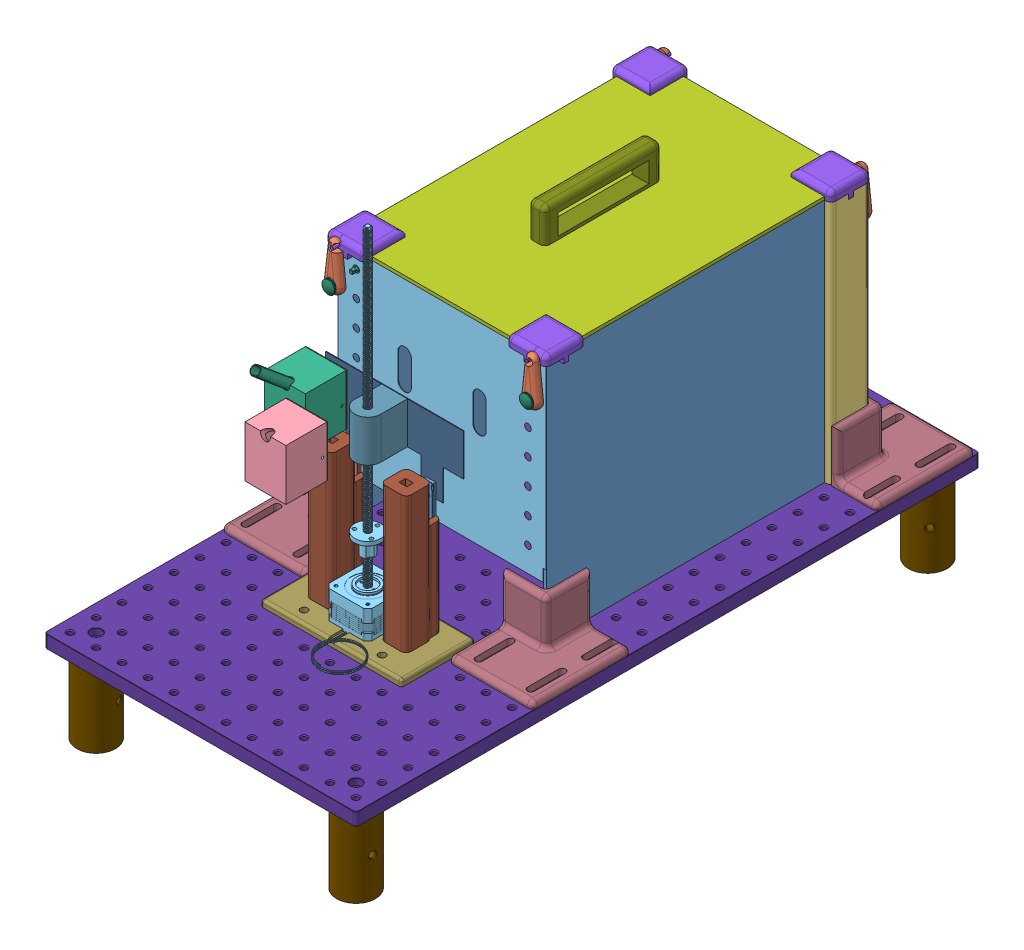
SolidWorks assembly Cage_model, configuration Default. Lengths in mm.
Overall size (306.09 428.48 610.88).
37 component instances, 27 part files, 73 mates.
Components (placement in the parent):
- Cage_acryllic_main-1: Cage_acryllic_main [Default] at (116.4275 -22.4186 -541.0136) size (203.2 239 304.17)
- Locking Mechanism^Cage_model-1: Locking Mechanism^Cage_model [Default] at (119.1314 -13.6836 -491.0988) x (0.989545 0 -0.144222) z (0.144222 0 0.989545) size (209.18 47.14 36.28) (virtual)
- Rear Legs^Cage_model-1: Rear Legs^Cage_model [Default] at (116.4275 -20.4186 -541.0136) x (0 0 -1) z (1 0 0) size (39.08 239 215.9) (virtual)
- Copy of Copy of Tube_Housing^Cage_model-1: Copy of Copy of Tube_Housing^Cage_model [Default] at (-6032.3573 5923.2833 -81.4233) size (40 50 40) (virtual)
- Stainless_steel_faceplate^Cage_model-1: Stainless_steel_faceplate^Cage_model [Default] at (116.4275 -20.4186 -236.8386) x (1 0 0) z (0 0 -1) size (203.2 188.94 0.61)
- Copy of Tube_Housing^Cage_model-2: Copy of Tube_Housing^Cage_model [Default] at (-6110.9268 5878.9507 -178.946) size (40 77.55 71.62) (virtual)
- cage top^Cage_model-1: cage top^Cage_model [Default] at (115.7745 -70.1218 -538.1595) size (203.2 3.18 304.78) (virtual)
- Top Securing Mechanisms-1: Top Securing Mechanisms [Default] at (-397.5627 136.2654 -668.6884) x (0 0 -1) z (0 1 0) size (45.43 215.9 14.36)
- doorMotorStand ^Cage_model-1: doorMotorStand ^Cage_model [Default] at (-254.8675 208.1203 679.8373) x (1 0 0) z (0 1 0) (virtual)
- Front legs^Cage_model-2: Front legs^Cage_model [Default] at (-86.7725 -20.4186 -236.229) x (0 0 1) z (-1 0 0) size (39.36 239 215.9) (hidden, virtual)
- Locking Mechanism^Cage_model-2: Locking Mechanism^Cage_model [Default] at (-90.3528 -13.1056 -286.1438) x (-0.989536 0.004347 0.144222) z (-0.144221 0.000634 -0.989545) size (209.18 47.14 36.28) (virtual)
- Top Securing Mechanisms-3: Top Securing Mechanisms [Default] at (427.2177 136.2654 -108.5542) x (0 0 1) z (0 1 0) size (45.43 215.9 14.36)
- Housing Door^Cage_model-1: Housing Door^Cage_model [Default] at (-6032.3573 5923.2833 -73.9233) x (-1 0 0) z (0 0 -1) size (40 50 0.61) (virtual)
- Door-2: Door [Default] at (467.6811 -160.8236 14.8493) x (0.996569 0.000281 -0.082761) z (-0.082738 -0.020299 -0.996365) size (134.22 71.08 12.57)
- Part6^Cage_model-4: Part6^Cage_model [Default] at (95.2928 -92.5203 546.9194) size (25.4 134.62 36.77) (virtual)
- Mounting Bracket nozzle holder-1: Mounting Bracket nozzle holder [Default] at (14.5275 -22.4186 -254) x (0 0 1) z (0 1 0) size (71.72 137.74 6.35)
- Angle Bracket_Leg Securing Mechanism-1: Angle Bracket_Leg Securing Mechanism [Default] at (156.2683 -22.4186 6.3564) x (1 0 0) z (0 1 0) size (304.2 433 50.8)
- Part6^Cage_model-5: Part6^Cage_model [Default] at (168.4928 -92.5203 546.8933) size (25.4 134.62 36.77) (virtual)
- Housing Door^Cage_model-2: Housing Door^Cage_model [Default] at (-6110.9268 5878.9507 -171.446) x (-1 0 0) z (0 0 -1) size (40 50 0.61) (virtual)
- Linear Motion Attachment Housing -2: Linear Motion Attachment Housing  [Default] at (68.2215 2233.7833 0) size (25.4 40.64 38.78)
- Part9^Cage_model-2: Part9^Cage_model [Default] at (239.0332 27.7971 -233.529) x (0.96536 0.260922 0) z (0 0 1) size (12.58 12.58 14.5) (virtual)
- Part9^Cage_model-1: Part9^Cage_model [Default] at (-93.8399 -16.6938 -233.529) x (0.891037 -0.453931 0) z (0 0 1) size (12.58 12.58 14.5) (virtual)
- Top Handle^Cage_model-1: Top Handle^Cage_model [Default] at (-0.1143 219.7614 179.188) x (1 0 0) z (0 1 0) size (16.56 114.3 33) (virtual)
- locking_mechanism^Cage_model-1: locking_mechanism^Cage_model [Default] at (0 0 310.525) (virtual)
- MB1224-Solidworks-1: MB1224-Solidworks [Default] at (14.5275 -35.1186 -304.8) x (0 0 1) z (-1 0 0) size (609.6 12.7 304.8)
- P3-Solidworks-1: P3-Solidworks [Web Part] at (-112.4725 -73.2186 -25.4) x (0.255609 0 0.96678) z (-0.96678 0 0.255609) size (37.74 76.2 37.94)
- P3-Solidworks-2: P3-Solidworks [Web Part] at (141.5275 -73.2186 -25.4) x (0.123275 0 -0.992373) z (0.992373 0 0.123275) size (37.74 76.2 37.94)
- P3-Solidworks-3: P3-Solidworks [Web Part] at (141.5275 -73.2186 -584.2) x (0.652104 0 -0.75813) z (0.75813 0 0.652104) size (37.74 76.2 37.94)
- P3-Solidworks-4: P3-Solidworks [Web Part] at (-112.4725 -73.2186 -584.2) x (-0.90982 0 0.415002) z (-0.415002 0 -0.90982) size (37.74 76.2 37.94)
- 3363N14_Miniature Pass-Through Drawer Slides-1: 3363N14_Miniature Pass-Through Drawer Slides [3363N14] at (51.1275 42.2414 -183.1224) x (0 1 0) z (0 0 -1) size (99.77 16 6)
- 3363N14_Miniature Pass-Through Drawer Slides (1)-1: 3363N14_Miniature Pass-Through Drawer Slides (1) [3363N14] at (-22.0725 42.2414 -183.0962) x (0 1 0) z (0 0 -1) size (99.77 16 6)
- 91028A658_JIS Hex Nut-1: 91028A658_JIS Hex Nut [91028A658] at (78.0275 -37.1186 -139.7) x (-0.777282 0 -0.629153) z (0.629153 0 -0.777282) size (8 4.57 9.24)
- 91028A658_JIS Hex Nut-4: 91028A658_JIS Hex Nut [91028A658] at (103.4275 -37.1186 -114.3) x (-0.799453 0 0.600729) z (-0.600729 0 -0.799453) size (8 4.57 9.24)
- LA1700-Solidworks-1: LA1700-Solidworks [Default] at (60.0219 191.9413 -69.6876) x (0 -0.690695 0.723146) z (-1 0 0) size (6 6 1.79)
- 8677N21_Stepper Motor with Linear Actuation-1: 8677N21_Stepper Motor with Linear Actuation [8677N21] at (14.5275 163.7634 -163.8403) x (0 -1 0) z (1 0 0) size (339.67 87.09 59.64)
- 91430A226_18-8 Stainless Steel Slotted Flat Head Screws (2)-1: 91430A226_18-8 Stainless Steel Slotted Flat Head Screws (2) [91430A226] at (-69.0425 51.5814 -357.659) x (0 0 1) z (0.105467 0.994423 0) size (16.28 7.5 7.43)
- 91430A226_18-8 Stainless Steel Slotted Flat Head Screws (2)-2: 91430A226_18-8 Stainless Steel Slotted Flat Head Screws (2) [91430A226] at (-69.0425 201.5814 -238.8065) x (0 0 1) z (-0.058058 -0.998313 0) size (16.28 7.5 7.43)
Mates (geometry in assembly coordinates):
- Front right post alignment to breadboard: coincident anti-aligned: plane of MB1224-Solidworks-1 through (-134.8725 -35.1186 -606.6) normal (0 -1 0); plane of P3-Solidworks-1 through (-112.4725 -35.1186 -25.4) normal (0 1 0)
- Rear left post hole alignement : concentric anti-aligned: circle of MB1224-Solidworks-1; circle of P3-Solidworks-3
- Rear right post hole alignment: concentric anti-aligned: circle of MB1224-Solidworks-1; circle of P3-Solidworks-4
- rear left post to breadboard: coincident anti-aligned: plane of MB1224-Solidworks-1 through (-134.8725 -35.1186 -606.6) normal (0 -1 0); plane of P3-Solidworks-3 through (141.5275 -35.1186 -584.2) normal (0 1 0)
- rear right post to breadboard: coincident anti-aligned: plane of MB1224-Solidworks-1 through (-134.8725 -35.1186 -606.6) normal (0 -1 0); plane of P3-Solidworks-4 through (-112.4725 -35.1186 -584.2) normal (0 1 0)
- Front right post hole alignment: concentric anti-aligned: circle of MB1224-Solidworks-1; circle of P3-Solidworks-1
- Coincident110: coincident anti-aligned: plane of Cage_acryllic_main-1 through (116.4275 -22.4186 -236.8386) normal (0 0 1); plane of Stainless_steel_faceplate^Cage_model-1 through (116.4275 -20.4186 -236.8386) normal (0 0 -1)
- Coincident111: coincident aligned: plane of Cage_acryllic_main-1 through (116.4275 -22.4186 -537.8386) normal (1 0 0); plane of Stainless_steel_faceplate^Cage_model-1 through (116.4275 216.5814 -236.229) normal (1 0 0)
- Coincident112: coincident aligned: plane of Cage_acryllic_main-1 through (116.4275 216.5814 -537.8386) normal (0 1 0); plane of Stainless_steel_faceplate^Cage_model-1 through (-86.7725 216.5814 -236.229) normal (0 1 0)
- Coincident115: coincident anti-aligned: plane of Stainless_steel_faceplate^Cage_model-1 through (116.4275 -20.4186 -236.229) normal (0 0 1); plane of Front legs^Cage_model-2 through (-86.7725 -20.4186 -236.229) normal (0 0 -1)
- Coincident116: coincident anti-aligned: plane of Cage_acryllic_main-1 through (116.4275 -22.4186 -537.8386) normal (1 0 0); plane of Front legs^Cage_model-2 through (116.4275 -20.4186 -236.229) normal (-1 0 0)
- Coincident124: coincident anti-aligned: plane of Cage_acryllic_main-1 through (116.4275 -22.4186 -541.0136) normal (0 0 -1); plane of Rear Legs^Cage_model-1 through (116.4275 -20.4186 -541.0136) normal (0 0 1)
- Coincident125: coincident anti-aligned: plane of Cage_acryllic_main-1 through (116.4275 -22.4186 -537.8386) normal (1 0 0); plane of Rear Legs^Cage_model-1 through (116.4275 -20.4186 -541.0136) normal (-1 0 0)
- Coincident127: coincident anti-aligned: plane of Cage_acryllic_main-1 through (116.4275 216.5814 -537.8386) normal (0 1 0); plane of cage top^Cage_model-1 through (115.7745 216.5814 -538.1595) normal (0 -1 0)
- Parallel2: parallel aligned: plane of MB1224-Solidworks-1 through (-137.8725 -22.4186 -606.6) normal (-1 0 0); plane of Front legs^Cage_model-2 through (-93.1225 -20.4186 -236.229) normal (-1 0 0)
- Coincident130: coincident aligned: plane of Cage_acryllic_main-1 through (116.4275 -22.4186 -537.8386) normal (1 0 0); plane of cage top^Cage_model-1 through (116.4275 219.7614 -541.0136) normal (1 0 0)
- Coincident131: coincident aligned: plane of Stainless_steel_faceplate^Cage_model-1 through (116.4275 -20.4186 -236.229) normal (0 0 1); plane of cage top^Cage_model-1 through (-86.7725 219.7614 -236.229) normal (0 0 1)
- Coincident133: coincident aligned: plane of Rear Legs^Cage_model-1 through (122.7775 -20.4186 -541.0136) normal (1 0 0); plane of Top Securing Mechanisms-1 through (122.7775 281.3795 -668.6884) normal (1 0 0)
- Coincident134: coincident aligned: plane of Rear Legs^Cage_model-1 through (116.4275 -20.4186 -547.3636) normal (0 0 -1); plane of Top Securing Mechanisms-1 through (-397.5627 281.3795 -547.3636) normal (0 0 -1)
- Coincident136: coincident anti-aligned: plane of Front legs^Cage_model-2 through (122.7775 216.5814 -236.229) normal (0 1 0); plane of Top Securing Mechanisms-3 through (-397.5627 216.5814 -108.5542) normal (0 -1 0)
- Coincident137: coincident aligned: plane of Front legs^Cage_model-2 through (122.7775 -20.4186 -236.229) normal (1 0 0); plane of Top Securing Mechanisms-3 through (122.7775 281.3795 -108.5542) normal (1 0 0)
- Lock1: lock: 
- Lock2: lock: 
- Coincident234: coincident aligned: plane of MB1224-Solidworks-1 through (-134.8725 -22.4186 0) normal (0 0 1)
- Coincident253: coincident anti-aligned: plane of Copy of Tube_Housing^Cage_model-2 through (-6110.9268 5878.9507 -171.446) normal (0 0 -1); plane of Housing Door^Cage_model-2 through (-6110.9268 5878.9507 -171.446) normal (0 0 1)
- Coincident254: coincident aligned: plane of Copy of Tube_Housing^Cage_model-2 through (-54.1526 175.7249 -131.446) normal (0 1 0); plane of Housing Door^Cage_model-2 through (-14.1526 175.7249 -172.0556) normal (0 1 0)
- Coincident255: coincident aligned: plane of Copy of Tube_Housing^Cage_model-2 through (-54.1526 175.7249 -131.446) normal (-1 0 0); plane of Housing Door^Cage_model-2 through (-54.1526 175.7249 -172.0556) normal (-1 0 0)
- Coincident258: coincident anti-aligned: plane of MB1224-Solidworks-1 through (-134.8725 -22.4186 -606.6) normal (0 1 0); plane of Mounting Bracket nozzle holder^Cage_model-1 through (14.5275 -22.4186 -254) normal (0 -1 0)
- Coincident272: coincident anti-aligned: plane of Front legs^Cage_model-2 through (122.7775 -20.4186 -236.229) normal (1 0 0); plane of Angle Bracket_Leg Securing Mechanism-1 through (122.7775 42.8936 -268.9599) normal (-1 0 0)
- Coincident273: coincident anti-aligned: plane of Front legs^Cage_model-2 through (116.4275 -20.4186 -229.879) normal (0 0 1); plane of Angle Bracket_Leg Securing Mechanism-1 through (122.7775 52.871 -229.879) normal (0 0 -1)
- Coincident274: coincident aligned: plane of MB1224-Solidworks-1 through (166.9275 -22.4186 -606.6) normal (1 0 0); plane of Angle Bracket_Leg Securing Mechanism-1 through (166.9275 42.8936 -268.9599) normal (1 0 0)
- Lock3: lock: 
- Parallel5: parallel aligned: plane of Part6^Cage_model-4 through (-9.3725 -53.9896 -152.1258) normal (0 0 1); plane of Part6^Cage_model-5 through (63.8275 -53.9896 -152.152) normal (0 0 1)
- Parallel6: parallel aligned: plane of MB1224-Solidworks-1 through (-134.8725 -22.4186 -606.6) normal (0 1 0)
- Parallel9: parallel aligned: plane of Stainless_steel_faceplate^Cage_model-1 through (-86.7725 216.5814 -236.229) normal (0 1 0); plane of 3363N14_Miniature Pass-Through Drawer Slides-1 through (55.7775 107.007 -185.6224) normal (0 1 0)
- Coincident295: coincident anti-aligned: plane of MB1224-Solidworks-1 through (-134.8725 -35.1186 -606.6) normal (0 -1 0); plane of 91028A658_JIS Hex Nut-1 through (78.0275 -35.1186 -139.7) normal (0 1 0)
- Coincident311: coincident aligned: plane of 3363N14_Miniature Pass-Through Drawer Slides-1 through (55.7775 107.007 -185.6224) normal (0 1 0); plane of 3363N14_Miniature Pass-Through Drawer Slides (1)-1 through (-17.4225 107.007 -185.5962) normal (0 1 0)
- Coincident312: coincident anti-aligned: plane of Part6^Cage_model-5 through (61.7475 7.2414 -210.1867) normal (0 1 0); plane of 3363N14_Miniature Pass-Through Drawer Slides-1 through (59.1275 7.2414 -188.1224) normal (0 -1 0)
- Coincident313: coincident anti-aligned: plane of Part6^Cage_model-5 through (59.1275 -40.1591 -183.1224) normal (-1 0 0); plane of 3363N14_Miniature Pass-Through Drawer Slides-1 through (59.1275 7.2414 -188.1224) normal (1 0 0)
- Coincident3252: coincident aligned: plane of Front legs^Cage_model-2 through (116.4275 -20.4186 -229.879) normal (0 0 1); plane of Top Securing Mechanisms-3 through (-397.5627 281.3795 -229.879) normal (0 0 1)
- Coincident3257: coincident anti-aligned: plane of MB1224-Solidworks-1 through (-134.8725 -35.1186 -606.6) normal (0 -1 0); plane of 91028A658_JIS Hex Nut-4 through (103.4275 -35.1186 -114.3) normal (0 1 0)
- Concentric668: concentric anti-aligned: circle of MB1224-Solidworks-1; circle of P3-Solidworks-2
- Coincident3267: coincident anti-aligned: plane of MB1224-Solidworks-1 through (-134.8725 -35.1186 -606.6) normal (0 -1 0); plane of P3-Solidworks-2 through (141.5275 -35.1186 -25.4) normal (0 1 0)
- Lock7: lock: 
- Lock8: lock: 
- Coincident3292: coincident aligned: plane of Cage_acryllic_main-1 through (116.4275 216.5814 -537.8386) normal (0 1 0); plane of Front legs^Cage_model-2 through (-93.1225 216.5814 -236.229) normal (0 1 0)
- Coincident3293: coincident aligned: plane of Front legs^Cage_model-2 through (83.6975 -22.4186 -275.3602) normal (0 -1 0); plane of Angle Bracket_Leg Securing Mechanism-1 through (156.2683 -22.4186 6.3564) normal (0 -1 0)
- Coincident3297: coincident anti-aligned: plane of Angle Bracket_Leg Securing Mechanism-1 through (-126.6133 -22.4186 6.3564) normal (0 -1 0); plane of MB1224-Solidworks-1 through (-134.8725 -22.4186 -606.6) normal (0 1 0)
- Concentric681: concentric anti-aligned: circle of Front legs^Cage_model-2; cylinder of Part9^Cage_model-2 through (111.3475 187.1174 -209.3869) axis (0 0 -1) radius 5
- Tangent3: tangent anti-aligned: plane of Locking Mechanism^Cage_model-2 through (111.3513 186.8113 -223.529) normal (0 0 1); torus of Part9^Cage_model-2
- Concentric682: concentric anti-aligned: circle of Front legs^Cage_model-2; cylinder of Part9^Cage_model-1 through (-81.6925 187.1174 -209.3869) axis (0 0 -1) radius 5
- Tangent4: tangent anti-aligned: plane of Locking Mechanism^Cage_model-2 through (-81.6869 187.6593 -223.529) normal (0 0 1); torus of Part9^Cage_model-1
- Coincident3305: coincident aligned: plane of Door-2 through (-32.6925 122.3934 -189.9191) normal (-1 0 0); plane of Part6^Cage_model-4 through (-32.6925 7.2414 -210.1605) normal (-1 0 0)
- Coincident3308: coincident aligned: plane of Door-2 through (-52.6315 163.0334 -189.9191) normal (0 1 0); plane of Part8^Cage_model-2 through (14.5275 163.0334 -163.8403) normal (0 1 0)
- Coincident3309: coincident anti-aligned: plane of MB1224-Solidworks-1 through (-134.8725 -22.4186 -606.6) normal (0 1 0); plane of 8677N21_Stepper Motor with Linear Actuation-1 through (14.5275 -22.4186 -163.8403) normal (0 -1 0)
- Coincident3313: coincident anti-aligned: plane of Mounting Bracket nozzle holder^Cage_model-1 through (-6.5672 -22.4186 -184.935) normal (1 0 0); plane of 8677N21_Stepper Motor with Linear Actuation-1 through (-6.5672 11.3634 -163.8403) normal (-1 0 0)
- Coincident3314: coincident anti-aligned: plane of Mounting Bracket nozzle holder^Cage_model-1 through (35.6222 -22.4186 -184.935) normal (0 0 1); plane of 8677N21_Stepper Motor with Linear Actuation-1 through (14.5275 11.3634 -184.935) normal (0 0 -1)
- Concentric685: concentric aligned: cylinder of Part8^Cage_model-2 through (14.5275 112.4939 -163.8403) axis (0 1 0) radius 3.5; cone of 8677N21_Stepper Motor with Linear Actuation-1 through (14.5275 314.9728 -163.8403) axis (0 1 0)
- Concentric686: concentric anti-aligned: cylinder of Part8^Cage_model-2 through (22.7764 128.3934 -159.0778) axis (0 -1 0) radius 1.778; circle of 8677N21_Stepper Motor with Linear Actuation-1
- Coincident3317: coincident anti-aligned: plane of Door-2 through (467.6811 -160.8236 -189.9191) normal (0 0 1); plane of Part8^Cage_model-2 through (467.6811 568.902 -189.9191) normal (0 0 -1)
- Coincident3318: coincident anti-aligned: plane of Part6^Cage_model-4 through (-30.0725 -40.1591 -183.0962) normal (0 0 -1); plane of 3363N14_Miniature Pass-Through Drawer Slides (1)-1 through (-30.0725 7.2414 -183.0962) normal (0 0 1)
- Coincident3319: coincident anti-aligned: plane of Part6^Cage_model-4 through (-30.0725 -40.1591 -183.0962) normal (1 0 0); plane of 3363N14_Miniature Pass-Through Drawer Slides (1)-1 through (-30.0725 7.2414 -188.0962) normal (-1 0 0)
- Coincident3320: coincident anti-aligned: plane of Part6^Cage_model-5 through (43.1275 -40.1591 -183.1224) normal (0 0 -1); plane of 3363N14_Miniature Pass-Through Drawer Slides-1 through (43.1275 7.2414 -183.1224) normal (0 0 1)
- Concentric692: concentric anti-aligned: circle of Copy of Tube_Housing^Cage_model-1; circle of LA1700-Solidworks-1
- Coincident3321: coincident anti-aligned: plane of Copy of Copy of Tube_Housing^Cage_model-1 through (-6032.3573 5923.2833 -73.9233) normal (0 0 -1); plane of Housing Door^Cage_model-1 through (-6032.3573 5923.2833 -73.9233) normal (0 0 1)
- Coincident3322: coincident aligned: plane of Copy of Copy of Tube_Housing^Cage_model-1 through (64.4169 220.0575 -33.9233) normal (1 0 0); plane of Housing Door^Cage_model-1 through (64.4169 220.0575 -74.5329) normal (1 0 0)
- Coincident3323: coincident aligned: plane of Copy of Copy of Tube_Housing^Cage_model-1 through (24.4169 220.0575 -33.9233) normal (0 1 0); plane of Housing Door^Cage_model-1 through (64.4169 220.0575 -74.5329) normal (0 1 0)
- Coincident3327: coincident aligned: plane of Copy of Copy of Tube_Housing^Cage_model-1 through (60.9169 191.9413 -69.6876) normal (-1 0 0); circle of LA1700-Solidworks-1
- Coincident3328: coincident: point of Cage_acryllic_main-1; plane of Rear Legs^Cage_model-1 through (122.7775 216.5814 -541.0136) normal (0 1 0)
- Coincident3329: coincident anti-aligned: plane of cage top^Cage_model-1 through (115.7745 219.7614 -538.1595) normal (0 1 0); plane of Top Handle^Cage_model-1 through (-0.1143 219.7614 179.188) normal (0 -1 0)
- Lock10: lock: 
- Coincident3330: coincident aligned: plane of Angle Bracket_Leg Securing Mechanism-1 through (166.9275 42.8936 -268.9599) normal (1 0 0); plane of MB1224-Solidworks-1 through (166.9275 -22.4186 -606.6) normal (1 0 0)
- Concentric695: concentric aligned: circle of Front legs^Cage_model-2; circle of 91430A226_18-8 Stainless Steel Slotted Flat Head Screws (2)-2
